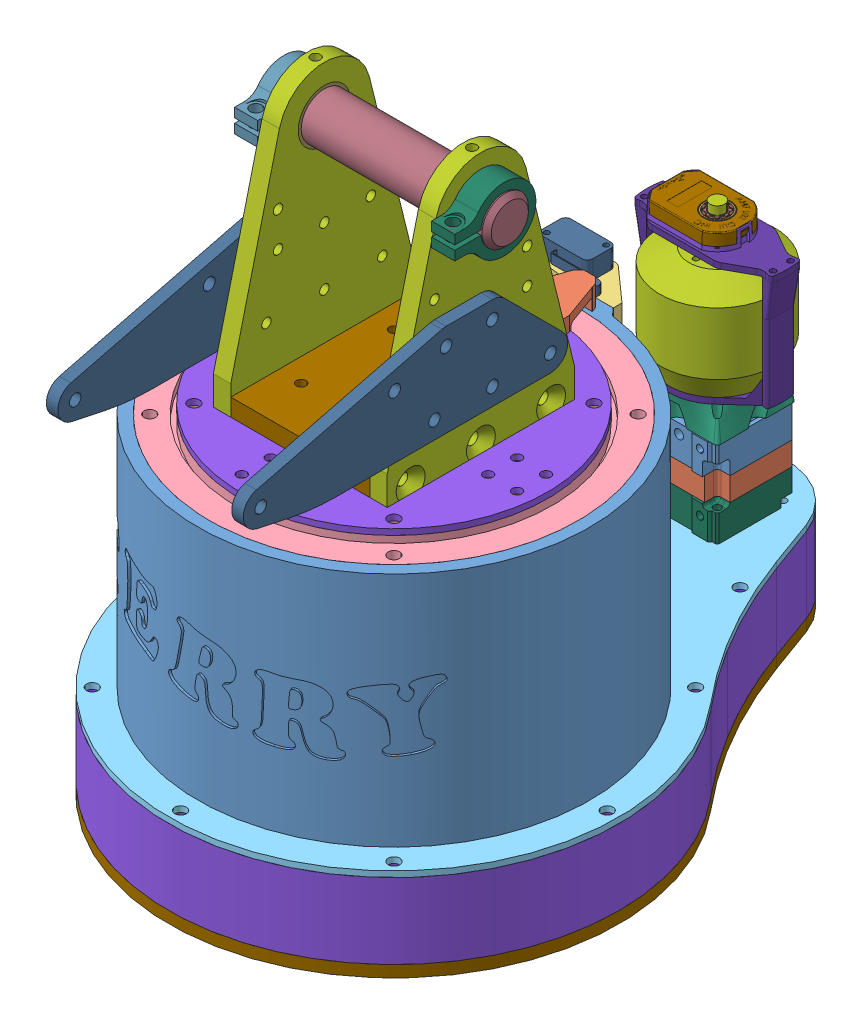
SolidWorks assembly Base, configuration Default. Lengths in mm.
Overall size (246.45 328.45 351.82).
86 component instances, 58 part files, 25 mates.
Components (placement in the parent):
- BotTurretHousing^Base-1: BotTurretHousing^Base [Default] at origin size (214.7 129.6 217.88) (virtual)
- SwitchTripper^Base-2: SwitchTripper^Base [Default] at origin size (28.57 11.52 54.14) (virtual)
- J1SwitchMount^Base-1: J1SwitchMount^Base [Default] at origin size (48.43 36.2 22.29) (virtual)
- 8in-1: 8in [Default] at (0 58.8 0) size (202 16 202)
- 8in-2: 8in [Default] at (0 -58.8 0) x (1 0 0) z (0 0 -1) size (202 16 202)
- BasePlate^Base-1: BasePlate^Base [Default] at origin size (246.45 3.17 338.52) (virtual)
- BotTurretPlate^Base-1: BotTurretPlate^Base [Default] at origin size (168.46 3.17 168.46) (virtual)
- SideTurretPlate^Base-1: SideTurretPlate^Base [Default] at origin size (9.52 279.65 102.6) (virtual)
- SideTurretPlate^Base-3: SideTurretPlate^Base [Default] x (-1 0 0) z (0 0 -1) size (9.52 279.65 102.6) (virtual)
- TopTurretPlate^Base-1: TopTurretPlate^Base [Default] at origin size (168.46 3.17 168.46) (virtual)
- TopBrace-1: TopBrace [Default] at origin size (76.2 9.53 102.6)
- PivotPlate^Base-1: PivotPlate^Base [Default] at origin size (6.35 50.8 177.8) (virtual)
- PivotPlate^Base-2: PivotPlate^Base [Default] at (101.6 0 0) size (6.35 50.8 177.8) (virtual)
- Keda9to1-1: Keda9to1 [Default] at (0 -48.175 -154.975) x (0 -1 0) z (1 0 0) size (176.96 63 76.93)
  - VersaPlanetary_v2_Single_Stage_10_1_with_BAG.STEP-1: VersaPlanetary_v2_Single_Stage_10_1_with_BAG.STEP [Default] at origin size (163.4 63.52 63.52)
    - 217-2820 Rev1_Public.STEP-1: 217-2820 Rev1_Public.STEP [Default] at (-4.6546 22.225 0) x (0 -0.456494 0.889726) z (-1 0 0) size (39.22 38.88 17.4)
      - 217-2625-100.STEP-1: 217-2625-100.STEP [Default] at origin size (39.22 38.88 12.7)
        - 217-2625-008 Rev1.STEP-1: 217-2625-008 Rev1.STEP [Default] at origin size (34.7 34.7 4.7)
        - 217-2625-010 Rev1.STEP-1: 217-2625-010 Rev1.STEP [Default] at (0 10.193 3.65) x (0.999813 0.019336 0) z (0 0 1) size (4 4 12)
        - 217-2625-010 Rev1.STEP-2: 217-2625-010 Rev1.STEP [Default] at (8.691 -5.3258 3.65) size (4 4 12)
        - 217-2625-010 Rev1.STEP-3: 217-2625-010 Rev1.STEP [Default] at (-8.691 -5.3258 3.65) size (4 4 12)
        - 217-2625-005 Rev1_Planet_Revolving_Follower01.STEP-1: 217-2625-005 Rev1_Planet_Revolving_Follower01.STEP [Default] at (8.691 -5.3258 6.35) x (0.932816 0.360354 0) z (0 0 1) size (16.89 16.89 8)
        - 217-2625-005 Rev1_Planet_Revolving_Follower01.STEP-2: 217-2625-005 Rev1_Planet_Revolving_Follower01.STEP [Default] at (-8.691 -5.3258 6.35) x (-0.932788 -0.360426 0) z (0 0 1) size (16.89 16.89 8)
        - 217-2625-005 Rev1_Planet_Revolving_Follower01.STEP-3: 217-2625-005 Rev1_Planet_Revolving_Follower01.STEP [Default] at (0 10.193 6.35) x (0.893583 0.448898 0) z (0 0 1) size (16.89 16.89 8)
      - 217-2625-007 Rev1_Public.STEP-1: 217-2625-007 Rev1_Public.STEP [Default] at (0 0 6.7) x (0.992772 0.120019 0) z (0 0 1) size (15.27 15.27 12.7)
    - 217-2625-026 Rev1.STEP-1: 217-2625-026 Rev1.STEP [Default] at (-6.5 22.225 0) x (0 -1 0) z (-1 0 0) size (44.45 42 18.12)
    - 217-2742-001 Rev4.STEP-1: 217-2742-001 Rev4.STEP [Default] at (0.2002 22.225 0) x (1 0 0) z (0 -0.092627 0.995701) size (7 28 28)
    - 217-2742-001 Rev4.STEP-2: 217-2742-001 Rev4.STEP [Default] at (8.2002 22.225 0) size (7 28 28)
    - 217-2625-017 Rev1_9714K61.STEP-1: 217-2625-017 Rev1_9714K61.STEP [Default] at (7.42 22.3002 -0.342) x (0 0.56703 0.823697) z (0 -0.823697 0.56703) size (28.51 4.98 27.43)
    - 217-2625-003 Rev1.STEP-1: 217-2625-003 Rev1.STEP [Default] at (7.4478 22.225 0) x (0 -1 0) z (1 0 0) size (17 17 64.11) (hidden)
    - 217-2625-018 Rev1_98541A410.STEP-1: 217-2625-018 Rev1_98541A410.STEP [Default] at (-0.7046 22.225 0) x (1 0 0) z (0 -0.017452 0.999848) size (1 19.6 17.4)
    - 832-1750-Ring-Gear-Screw_SSA0832-0500ZC.STEP-1: 832-1750-Ring-Gear-Screw_SSA0832-0500ZC.STEP [Default] at (-30.7 4.725 -17.5) x (0 0.997447 0.071411) z (0 -0.071411 0.997447) size (6.73 48.51 6.73) (hidden)
    - 832-1750-Ring-Gear-Screw_SSA0832-0500ZC.STEP-2: 832-1750-Ring-Gear-Screw_SSA0832-0500ZC.STEP [Default] at (-30.7 39.725 17.5) x (0 0.005929 0.999982) z (0 -0.999982 0.005929) size (6.73 48.51 6.73) (hidden)
    - 217-2625-025 Rev1.STEP-1: 217-2625-025 Rev1.STEP [Default] at (-23.2 22.225 0) x (0 -1 0) z (-1 0 0) size (44.45 42 18)
    - 217-4649-002 Rev1_SSA0832-0500ZC.STEP-1: 217-4649-002 Rev1_SSA0832-0500ZC.STEP [Default] at (-33.7 4.2645 17.9605) x (0 0.33842 -0.940995) z (0 0.940995 0.33842) size (6.73 16.76 6.73) (hidden)
    - 217-4649-002 Rev1_SSA0832-0500ZC.STEP-2: 217-4649-002 Rev1_SSA0832-0500ZC.STEP [Default] at (-33.7 40.1855 -17.9605) x (0 -0.308932 -0.951084) z (0 0.951084 -0.308932) size (6.73 16.76 6.73) (hidden)
    - 217-4649-006 Rev1_SSA0004-008BA.STEP-1: 217-4649-006 Rev1_SSA0004-008BA.STEP [Default] at (-30.7 22.225 12.5) x (0 0.5 -0.866025) z (0 -0.866025 -0.5) size (7 14 7) (hidden)
    - 217-4649-006 Rev1_SSA0004-008BA.STEP-2: 217-4649-006 Rev1_SSA0004-008BA.STEP [Default] at (-30.7 22.225 -12.5) x (0 -0.5 0.866025) z (0 0.866025 0.5) size (7 14 7) (hidden)
    - 217-2822-003 Rev4.STEP-1: 217-2822-003 Rev4.STEP [Default] at (-32.2 22.225 0) x (0 -1 0) z (-1 0 0) size (42 42 4.8) (hidden)
    - 217-3351 Rev2.STEP-1: 217-3351 Rev2.STEP [Default] at (-33.7 22.225 0) x (0 0 1) z (1 0 0) size (59.07 59.07 84.5) (hidden)
    - 217-2816-001 Rev1.STEP-1: 217-2816-001 Rev1.STEP [Default] at (-6.35 22.225 0) x (0 -1 0) z (1 0 0) size (42 42 14.51)
    - 217-4649-001 Rev1.STEP-1: 217-4649-001 Rev1.STEP [Default] at (-20.046 22.225 0) x (0 -1 0) z (1 0 0) size (18 18 13)
    - 217-4649-007 Rev1_94105A824.STEP-1: 217-4649-007 Rev1_94105A824.STEP [Default] at (-25.521 22.225 -6.7835) x (-0.996104 -0.088191 0) z (0 0 -1) size (4.83 4.83 4.77)
    - 217-2625-011 Rev1.STEP-1: 217-2625-011 Rev1.STEP [Default] at (-24.7818 22.225 0) x (0 0 1) z (0 -1 0) size (8.01 7.5 7.94) (hidden)
  - VersaPlanetary_CIM_Motor_Output_Shaft_Kit_217-2893-1: VersaPlanetary_CIM_Motor_Output_Shaft_Kit_217-2893 [Default] at (7.4478 22.225 0) x (0 0 -1) z (1 0 0) size (17 17 57.85)
  - KedaAdapter^Keda9to1-1: KedaAdapter^Keda9to1 [Default] at origin size (17.82 53.01 53.01) (virtual)
  - 192kvMotorEncoded-1: 192kvMotorEncoded [Default] at (-51.0318 22.225 0) x (0 -1 0) z (0 0 -1) size (63 104.52 76.93)
    - BetterKEDA-1: BetterKEDA [Default] at origin size (63 104.52 63)
    - CUI_DEVICES_AMT102-0048-N2000-S-1: CUI_DEVICES_AMT102-0048-N2000-S [Default] at (0 65.12 0) x (1 0 0) z (0 1 0) size (36.33 46.21 9.2)
      - CUI_DEVICES_AMT102-0048-N2000-S.step-1: CUI_DEVICES_AMT102-0048-N2000-S.step [Default] at origin size (36.33 46.21 9.2)
        - AMT-102-Base-REV-K.step-1: AMT-102-Base-REV-K.step [Default] x (-1 0 0) z (0 0 -1) size (28.78 43.39 9.06)
        - AMT-102-Top-Cover-REV-H.step-1: AMT-102-Top-Cover-REV-H.step [Default] at (0 0 5.23) x (-1 0 0) z (0 0 -1) size (28.6 43.26 6.55)
        - AMT-Sleeve-REV-D_ 2 mm.step-1: AMT-Sleeve-REV-D_ 2 mm.step [Default] at (0 0 -2.42) x (0.999996 0.002864 0) z (0 0 1) size (10.79 10.79 7.8)
        - AMT-Hub-Top-REV-D1.step-1: AMT-Hub-Top-REV-D1.step [Default] at (0 0 2.13) x (0.999996 0.002864 0) z (0 0 1) size (14 14 5.67)
        - AMT-Hub-Bottom-REV-B.step-1: AMT-Hub-Bottom-REV-B.step [Default] at (0 0 2.43) x (0.999998 -0.001942 0) z (0 0 1) size (17.3 17.3 3.2)
        - AMT10X-Shaft-Adaptor-REV-E.step-1: AMT10X-Shaft-Adaptor-REV-E.step [Default] at (0 0 0.03) x (0.999996 0.002864 0) z (0 0 1) size (11.8 11.8 7.8)
        - Receiver-board.step-1: Receiver-board.step [Default] at (72.2834 -20.351 3.03) x (-1 0 0) z (0 0 -1) size (26.5 26.62 0.41)
        - Rotor-board-REV F.step-1: Rotor-board-REV F.step [Default] at (0 0 2.13) x (0.807874 -0.589355 0) z (0 0 1) size (26 26 0.3)
        - Transmitter-board AMT10_AMT-102.step-1: Transmitter-board AMT10_AMT-102.step [Default] at (19.1596 -17.1102 1.22) x (-1 0 0) z (0 0 -1) size (26.63 38.43 4.41)
    - Body^192kvMotorEncoded-1: Body^192kvMotorEncoded [Default] at origin size (53 64.53 76.93) (virtual)
- J1Pulley-1: J1Pulley [Default] at (0 -94.5 0) size (144.9 24.53 144.9)
- 15Tpulley-2: 15Tpulley [Default] at (0 -86.5 -177.2) size (28 28 28)
- J1Belt133T^Base-1: J1Belt133T^Base [Default] at origin size (148.26 15.01 264.1) (virtual)
- TensionPillarJ1-1: TensionPillarJ1 [Default] at (5.0959 -4.9525 -9.5995) size (38.1 25.73 38.1)
  - 98019A228_MIL SPEC. 300 SERIES SS FLAT WASHER-1: 98019A228_MIL SPEC. 300 SERIES SS FLAT WASHER [98019A228] at (20.3041 -73.2587 -110.4505) x (0.972939 0 -0.231063) z (0.231063 0 0.972939) size (9.53 0.71 9.53)
  - 60355K701_BALL BEARING-1: 60355K701_BALL BEARING [60355K701] at (20.3041 -75.7479 -110.4505) x (1 0 0) z (0 1 0) size (15.88 15.88 4.98)
  - Roller^TensionPillarJ1-1: Roller^TensionPillarJ1 [Default] at (-2.0675 -15.5777 2.6827) size (38.1 15.96 38.1) (virtual)
  - 60355K701_BALL BEARING-2: 60355K701_BALL BEARING [60355K701] at (20.3041 -86.2673 -110.4505) x (1 0 0) z (0 1 0) size (15.88 15.88 4.98)
  - 375spacer-1: 375spacer [92510A777] at (20.3041 -67.785 -110.4505) x (1 0 0) z (0 -1 0) size (15.88 15.88 9.53)
- TensionPillarJ1-2: TensionPillarJ1 [Default] at (-5.0959 -4.9525 -230.5005) x (-1 0 0) z (0 0 -1) size (38.1 25.73 38.1)
  - 98019A228_MIL SPEC. 300 SERIES SS FLAT WASHER-1: 98019A228_MIL SPEC. 300 SERIES SS FLAT WASHER [98019A228] at (20.3041 -73.2587 -110.4505) x (0.972939 0 -0.231063) z (0.231063 0 0.972939) size (9.53 0.71 9.53)
  - 60355K701_BALL BEARING-1: 60355K701_BALL BEARING [60355K701] at (20.3041 -75.7479 -110.4505) x (1 0 0) z (0 1 0) size (15.88 15.88 4.98)
  - Roller^TensionPillarJ1-1: Roller^TensionPillarJ1 [Default] at (-2.0675 -15.5777 2.6827) size (38.1 15.96 38.1) (virtual)
  - 60355K701_BALL BEARING-2: 60355K701_BALL BEARING [60355K701] at (20.3041 -86.2673 -110.4505) x (1 0 0) z (0 1 0) size (15.88 15.88 4.98)
  - 375spacer-1: 375spacer [92510A777] at (20.3041 -67.785 -110.4505) x (1 0 0) z (0 -1 0) size (15.88 15.88 9.53)
- TensionConnector^Base-1: TensionConnector^Base [Default] at origin size (66.67 5.72 15.88) (virtual)
- Foot^Base-1: Foot^Base [Default] at origin size (246.45 41.28 338.52) (virtual)
- Sole^Base-1: Sole^Base [Default] at origin size (246.45 6.35 338.52) (virtual)
- switch-1: switch [Default] at (-34 69.95 -117.75) x (-1 0 0) z (0 0 -1) size (39.3 10.3 27.5)
- 94459A340_BRASS HEAT-SET INSERT FOR PLASTIC-1: 94459A340_BRASS HEAT-SET INSERT FOR PLASTIC [94459A340] at (0 52.1 -104.175) x (0.708984 0.705225 0) z (-0.705225 0.708984 0) size (7.22 6.55 7.22)
- 94459A340_BRASS HEAT-SET INSERT FOR PLASTIC-2: 94459A340_BRASS HEAT-SET INSERT FOR PLASTIC [94459A340] at (0 39.4 -104.175) x (0.708984 0.705225 0) z (-0.705225 0.708984 0) size (7.22 6.55 7.22)
- 6391K422_OIL-EMBEDDED SLEEVE BEARING-1: 6391K422_OIL-EMBEDDED SLEEVE BEARING [6391K422] at (-44.45 187.45 0) x (0 0 -1) z (1 0 0) size (28.63 28.63 12.7)
- 6061K603_HARDENED PRECISION STEEL SHAFT-1: 6061K603_HARDENED PRECISION STEEL SHAFT [6061K603] at (0 187.45 0) size (127 25.4 25.4)
- 6391K422_OIL-EMBEDDED SLEEVE BEARING-2: 6391K422_OIL-EMBEDDED SLEEVE BEARING [6391K422] at (44.45 187.45 0) x (0 0 -1) z (1 0 0) size (28.63 28.63 12.7)
- SideClamp-1: SideClamp [Default] at origin size (12.7 34.92 44.45)
- MirrorSideClamp-3: MirrorSideClamp [Default] x (-1 0 0) z (0 0 -1) size (12.7 34.92 44.45)
Mates (geometry in assembly coordinates):
- Concentric1: concentric aligned: cylinder of BotTurretHousing^Base-1 through (0 50.8 0) axis (0 -1 0) radius 86.77; cylinder of 8in-1 through (0 64.8 0) axis (0 -1 0) radius 70
- Coincident1: coincident anti-aligned: plane of BotTurretHousing^Base-1 through (0 50.8 0) normal (0 1 0); plane of 8in-1 through (0 50.8 0) normal (0 -1 0)
- Concentric4: concentric anti-aligned: cylinder of BasePlate^Base-1 through (0 -67.975 -177.2) axis (0 1 0) radius 10; cylinder of Keda9to1-1/VersaPlanetary_CIM_Motor_Output_Shaft_Kit_217-2893-1 through (0 -63.3752 -177.2) axis (0 -1 0) radius 8.5
- Concentric5: concentric aligned: cylinder of BasePlate^Base-1 through (17.9605 -67.975 -159.2395) axis (0 1 0) radius 1.9844; cylinder of Keda9to1-1/VersaPlanetary_v2_Single_Stage_10_1_with_BAG.STEP-1/217-2625-026 Rev1.STEP-1 through (17.9605 -48.175 -159.2395) axis (0 1 0) radius 2.0193
- Coincident2: coincident anti-aligned: plane of BasePlate^Base-1 through (0 -64.8 0) normal (0 1 0); plane of Keda9to1-1/VersaPlanetary_v2_Single_Stage_10_1_with_BAG.STEP-1/217-2625-026 Rev1.STEP-1 through (22.225 -64.8 -199.425) normal (0 -1 0)
- Coincident3: coincident aligned: plane of J1Pulley-1 through (0 -94.5 0) normal (0 0 1)
- Coincident4: coincident aligned: plane of J1Pulley-1 through (0 -94.5 0) normal (1 0 0)
- Coincident7: coincident anti-aligned: plane of BotTurretPlate^Base-1 through (0 -69.975 0) normal (0 -1 0); plane of J1Pulley-1 through (0 -69.975 0) normal (0 1 0)
- Concentric6: concentric anti-aligned: cylinder of Keda9to1-1/VersaPlanetary_CIM_Motor_Output_Shaft_Kit_217-2893-1 through (0 -141.9432 -177.2) axis (0 1 0) radius 3.975; cylinder of 15Tpulley-2 through (0 -78.5 -177.2) axis (0 -1 0) radius 4
- Coincident8: coincident anti-aligned: plane of J1Pulley-1 through (0 -94.5 0) normal (0 -1 0); plane of 15Tpulley-2 through (0 -94.5 -177.2) normal (0 1 0)
- Concentric13: concentric anti-aligned: cylinder of BotTurretHousing^Base-1 through (0 52.1 107.3573) axis (0 0 -1) radius 3.2639; cylinder of 94459A340_BRASS HEAT-SET INSERT FOR PLASTIC-1 through (0 52.1 -104.175) axis (0 0 1) radius 3.1623
- Coincident15: coincident aligned: plane of BotTurretHousing^Base-1 through (0 39.4 -110.525) normal (0 0 -1); plane of 94459A340_BRASS HEAT-SET INSERT FOR PLASTIC-1 through (2.5211 54.6078 -110.525) normal (0 0 -1)
- Concentric14: concentric anti-aligned: cylinder of BotTurretHousing^Base-1 through (0 39.4 107.3573) axis (0 0 -1) radius 3.2639; cylinder of 94459A340_BRASS HEAT-SET INSERT FOR PLASTIC-2 through (0 39.4 -104.175) axis (0 0 1) radius 3.1623
- Coincident16: coincident aligned: plane of BotTurretHousing^Base-1 through (0 39.4 -110.525) normal (0 0 -1); plane of 94459A340_BRASS HEAT-SET INSERT FOR PLASTIC-2 through (2.5211 41.9078 -110.525) normal (0 0 -1)
- Parallel1: parallel anti-aligned: plane of BotTurretHousing^Base-1 through (0 64.8 0) normal (0 1 0); plane of switch-1 through (-34 64.8 -117.75) normal (0 -1 0)
- Coincident19: coincident: line of switch-1 through (0 72.45 -109.85) axis (0 -1 0)
- Parallel2: parallel aligned: plane of switch-1 through (-34 75.1 -114.95) normal (0 0 1)
- Tangent1: tangent anti-aligned: cylinder of BotTurretHousing^Base-1 through (0 368.4317 0) axis (0 -1 0) radius 107.35; cylinder of switch-1 through (0 72.45 -109.85) axis (0 -1 0) radius 2.5
- Coincident22: coincident anti-aligned: plane of BotTurretHousing^Base-1 through (0 64.8 0) normal (0 1 0); plane of switch-1 through (-34 64.8 -117.75) normal (0 -1 0)
- Coincident23: coincident aligned: plane of SideTurretPlate^Base-1 through (-38.1 187.45 0) normal (1 0 0); plane of 6391K422_OIL-EMBEDDED SLEEVE BEARING-1 through (-38.1 187.45 0) normal (1 0 0)
- Concentric16: concentric aligned: cylinder of SideTurretPlate^Base-1 through (-38.1 187.45 0) axis (-1 0 0) radius 14.3129; cylinder of 6391K422_OIL-EMBEDDED SLEEVE BEARING-1 through (-38.1 187.45 0) axis (-1 0 0) radius 12.7
- Concentric17: concentric anti-aligned: cylinder of 6391K422_OIL-EMBEDDED SLEEVE BEARING-1 through (-38.1 187.45 0) axis (-1 0 0) radius 12.7; cylinder of 6061K603_HARDENED PRECISION STEEL SHAFT-1 through (-63.5 187.45 0) axis (1 0 0) radius 12.7
- Width1: width anti-aligned: plane of 6061K603_HARDENED PRECISION STEEL SHAFT-1 through (63.5 187.45 0) normal (1 0 0); plane of 6061K603_HARDENED PRECISION STEEL SHAFT-1 through (-63.5 187.45 0) normal (-1 0 0); plane of SideTurretPlate^Base-1 through (-47.625 187.45 0) normal (-1 0 0); plane of SideTurretPlate^Base-3 through (47.625 187.45 0) normal (1 0 0)
- Coincident24: coincident anti-aligned: plane of BasePlate^Base-1 through (0 -67.975 0) normal (0 -1 0); plane of TensionPillarJ1-1/375spacer-1 through (25.4 -67.975 -120.05) normal (0 1 0)
- Concentric18: concentric aligned: circle of BasePlate^Base-1; cylinder of TensionPillarJ1-1/375spacer-1 through (25.4 -77.5 -120.05) axis (0 1 0) radius 7.9375
